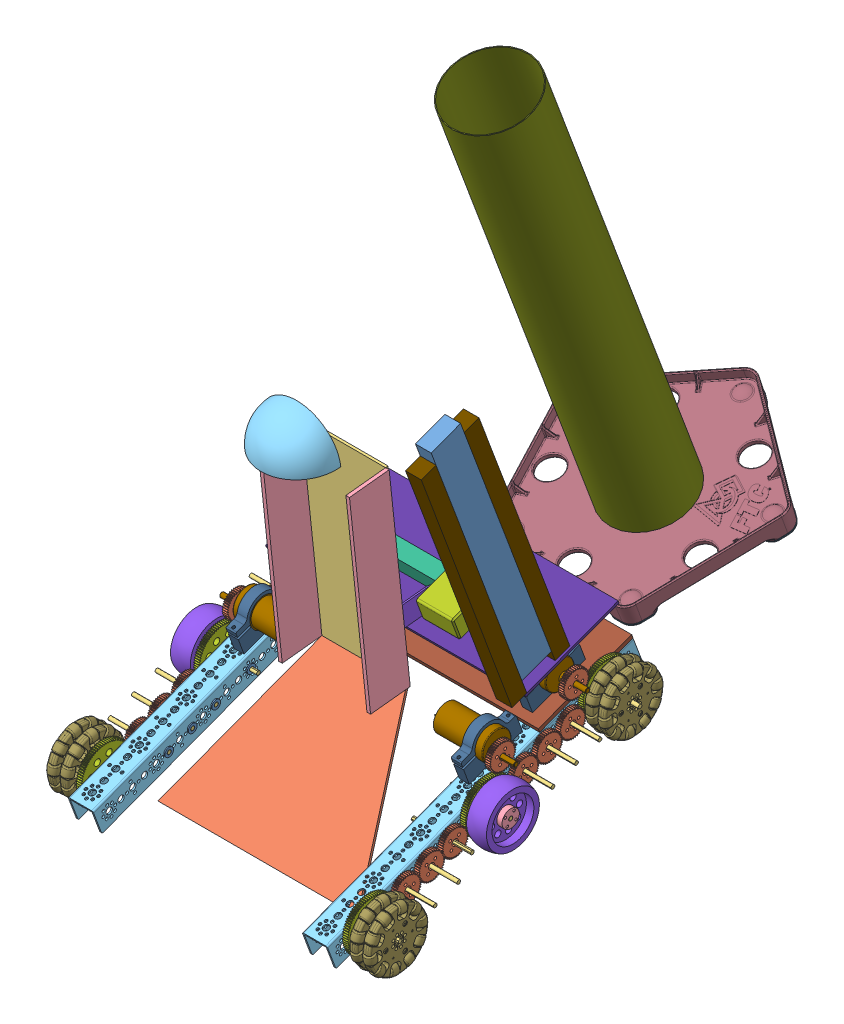
SolidWorks assembly 6157 - Basic Chassis, configuration Default. Lengths in mm.
Overall size (426.67 882.34 918.7).
152 component instances, 30 part files, 95 mates.
Components (placement in the parent):
- Part1^6157 - Basic Chassis-1: Part1^6157 - Basic Chassis [Default] at origin (virtual)
- ChassisSide^6157 - Basic Chassis-1: ChassisSide^6157 - Basic Chassis [Default] at (356.2135 -601.8803 193.3567) x (0 -0.61219 -0.790711) z (1 0 0) size (261.15 370.6 94.34) (virtual)
  - Copy of Assem7^ChassisSide_6157 - Basic Chassis-1: Copy of Assem7^ChassisSide_6157 - Basic Chassis [Default] at (59.0771 95.1521 -34.8) x (-0.863566 0.504235 0) z (0 0 -1) size (34.75 34.75 75.57) (virtual)
    - Axle bronze bushing-1: Axle bronze bushing [Default] at origin size (11 11 12.4)
    - Gear Metric 40T-1: Gear Metric 40T [PreviewCfg] at (0 0 -34.8) x (0 0 -1) z (0.99932 -0.03687 0) size (6.2 33.53 33.53)
    - Axle D-shaft-1: Axle D-shaft [Default] at (0 0 -37.7829) x (-0.991315 0.131508 0) z (0 0 1) size (4.73 4.46 75.57)
    - Axle bronze bushing-2: Axle bronze bushing [Default] at (0 0 -36.2) x (-0.381849 -0.924225 0) z (0 0 -1) size (11 11 12.4)
  - Hub axle shaft-1: Hub axle shaft [Default] at (0 0 25.25) x (-0.097328 0.995252 0) z (0 0 -1) size (22 22 9.5)
  - Pitsco Education-739069-1: Pitsco Education-739069 [Default] at (-109.4377 -176.8824 -17.4) x (0 0 1) z (-0.526143 -0.850396 0) size (32 32 416)
  - Axle bronze bushing-1: Axle bronze bushing [Default] at (-25.2548 -40.819 0) x (0.995682 -0.092835 0) z (0 0 1) size (11 11 12.4)
  - Axle bronze bushing-2: Axle bronze bushing [Default] at origin size (11 11 12.4)
  - Hub spacer-1: Hub spacer [Default] at (0 0 6.2) x (-0.466001 -0.884784 0) z (0 0 -1) size (22.2 22.2 17.7)
  - Axle D-shaft-1: Axle D-shaft [Default] at (0 0 -5.8329) x (0.055977 0.998432 0) z (0 0 1) size (4.73 4.46 75.57)
  - Gear Metric 80T-1: Gear Metric 80T [Metric - Spur gear 0.8M 80T 20PA 6.2FW ---S80N75H50L8.0N] x (0 0 1) z (-0.097328 0.995252 0) size (6.2 65.57 65.57)
  - Wheel 76mm 3-in-1: Wheel 76mm 3-in [Default] at (0 0 11.534) x (-0.995252 -0.097328 0) z (0 0 -1) size (72.2 72.2 25.4)
  - Axle bronze bushing-3: Axle bronze bushing [Default] at (0 0 -34.8) x (-0.466001 -0.884784 0) z (0 0 -1) size (11 11 12.4)
  - Axle bronze bushing-4: Axle bronze bushing [Default] at (-25.2548 -40.819 -34.8) x (-0.466001 -0.884784 0) z (0 0 -1) size (11 11 12.4)
  - Axle D-shaft-2: Axle D-shaft [Default] at (-25.2548 -40.819 -9.7171) x (0.055977 0.998432 0) z (0 0 1) size (4.73 4.46 75.57)
  - Gear Metric 40T-1: Gear Metric 40T [PreviewCfg] at (-25.2548 -40.819 0) x (0 0 1) z (0.013213 -0.999913 0) size (6.2 33.53 33.53)
  - Axle bronze bushing-5: Axle bronze bushing [Default] at (84.1828 136.0634 0) x (0.995682 -0.092835 0) z (0 0 1) size (11 11 12.4)
  - Copy of Assem7^ChassisSide_6157 - Basic Chassis-2: Copy of Assem7^ChassisSide_6157 - Basic Chassis [Default] at (-42.0914 -68.0317 -34.8) x (0.010961 -0.99994 0) z (0 0 -1) size (34.75 34.75 75.57) (virtual)
    - Axle bronze bushing-1: Axle bronze bushing [Default] at origin size (11 11 12.4)
    - Gear Metric 40T-1: Gear Metric 40T [PreviewCfg] at (0 0 -34.8) x (0 0 -1) z (0.99932 -0.03687 0) size (6.2 33.53 33.53)
    - Axle D-shaft-1: Axle D-shaft [Default] at (0 0 -37.7829) x (-0.991315 0.131508 0) z (0 0 1) size (4.73 4.46 75.57)
    - Axle bronze bushing-2: Axle bronze bushing [Default] at (0 0 -36.2) x (-0.381849 -0.924225 0) z (0 0 -1) size (11 11 12.4)
  - Gear Metric 80T-2: Gear Metric 80T [Metric - Spur gear 0.8M 80T 20PA 6.2FW ---S80N75H50L8.0N] at (84.1828 136.0634 0) x (0 0 1) z (-0.737059 -0.675828 0) size (6.2 65.57 65.57)
  - Axle D-shaft-3: Axle D-shaft [Default] at (84.1828 136.0634 9.0538) x (-0.905707 -0.423905 0) z (0 0 1) size (4.73 4.46 75.57)
  - Copy of OmniWheelGear^ChassisSide_6157 - Basic Chassis-1: Copy of OmniWheelGear^ChassisSide_6157 - Basic Chassis [Default] at (-84.1828 -136.0634 0) x (0.995682 -0.092835 0) z (0 0 1) size (92.61 92.61 75.57) (virtual)
    - Axle bronze bushing-1: Axle bronze bushing [Default] at origin size (11 11 12.4)
    - Axle bronze bushing-2: Axle bronze bushing [Default] at (0 0 -34.8) x (-0.381849 -0.924225 0) z (0 0 -1) size (11 11 12.4)
    - Axle D-shaft-1: Axle D-shaft [Default] at (0 0 2.9829) x (-0.596843 0.802358 0) z (0 0 1) size (4.73 4.46 75.57)
    - Gear Metric 80T-1: Gear Metric 80T [Metric - Spur gear 0.8M 80T 20PA 6.2FW ---S80N75H50L8.0N] x (0 0 1) z (-0.671136 -0.741335 0) size (6.2 65.57 65.57)
  - Copy of Assem7^ChassisSide_6157 - Basic Chassis-3: Copy of Assem7^ChassisSide_6157 - Basic Chassis [Default] at (-59.0771 -95.1521 -34.8) x (-0.863566 0.504235 0) z (0 0 -1) size (34.75 34.75 75.57) (virtual)
    - Axle bronze bushing-1: Axle bronze bushing [Default] at origin size (11 11 12.4)
    - Gear Metric 40T-1: Gear Metric 40T [PreviewCfg] at (0 0 -34.8) x (0 0 -1) z (0.99932 -0.03687 0) size (6.2 33.53 33.53)
    - Axle D-shaft-1: Axle D-shaft [Default] at (0 0 -37.7829) x (-0.991315 0.131508 0) z (0 0 1) size (4.73 4.46 75.57)
    - Axle bronze bushing-2: Axle bronze bushing [Default] at (0 0 -36.2) x (-0.381849 -0.924225 0) z (0 0 -1) size (11 11 12.4)
  - Copy of Assem7^ChassisSide_6157 - Basic Chassis-4: Copy of Assem7^ChassisSide_6157 - Basic Chassis [Default] at (42.0914 68.0317 -34.8) x (-0.863566 0.504235 0) z (0 0 -1) size (34.75 34.75 75.57) (virtual)
    - Axle bronze bushing-1: Axle bronze bushing [Default] at origin size (11 11 12.4)
    - Gear Metric 40T-1: Gear Metric 40T [PreviewCfg] at (0 0 -34.8) x (0 0 -1) z (0.99932 -0.03687 0) size (6.2 33.53 33.53)
    - Axle D-shaft-1: Axle D-shaft [Default] at (0 0 -37.7829) x (-0.991315 0.131508 0) z (0 0 1) size (4.73 4.46 75.57)
    - Axle bronze bushing-2: Axle bronze bushing [Default] at (0 0 -36.2) x (-0.381849 -0.924225 0) z (0 0 -1) size (11 11 12.4)
  - Copy of Assem7^ChassisSide_6157 - Basic Chassis-5: Copy of Assem7^ChassisSide_6157 - Basic Chassis [Default] at (25.2548 40.819 -34.8) x (-0.863566 0.504235 0) z (0 0 -1) size (34.75 34.75 75.57) (virtual)
    - Axle bronze bushing-1: Axle bronze bushing [Default] at origin size (11 11 12.4)
    - Gear Metric 40T-1: Gear Metric 40T [PreviewCfg] at (0 0 -34.8) x (0 0 -1) z (0.99932 -0.03687 0) size (6.2 33.53 33.53)
    - Axle D-shaft-1: Axle D-shaft [Default] at (0 0 -37.7829) x (-0.991315 0.131508 0) z (0 0 1) size (4.73 4.46 75.57)
    - Axle bronze bushing-2: Axle bronze bushing [Default] at (0 0 -36.2) x (-0.381849 -0.924225 0) z (0 0 -1) size (11 11 12.4)
- ChassisSide^6157 - Basic Chassis-2: ChassisSide^6157 - Basic Chassis [Default] at (23.2135 -601.8803 193.3567) x (0 -0.980825 0.194892) z (-1 0 0) size (261.15 370.6 94.34) (virtual)
  - Copy of Assem7^ChassisSide_6157 - Basic Chassis-1: Copy of Assem7^ChassisSide_6157 - Basic Chassis [Default] at (59.0771 95.1521 -34.8) x (-0.863566 0.504235 0) z (0 0 -1) size (34.75 34.75 75.57) (virtual)
    - Axle bronze bushing-1: Axle bronze bushing [Default] at origin size (11 11 12.4)
    - Gear Metric 40T-1: Gear Metric 40T [PreviewCfg] at (0 0 -34.8) x (0 0 -1) z (0.99932 -0.03687 0) size (6.2 33.53 33.53)
    - Axle D-shaft-1: Axle D-shaft [Default] at (0 0 -37.7829) x (-0.991315 0.131508 0) z (0 0 1) size (4.73 4.46 75.57)
    - Axle bronze bushing-2: Axle bronze bushing [Default] at (0 0 -36.2) x (-0.381849 -0.924225 0) z (0 0 -1) size (11 11 12.4)
  - Hub axle shaft-1: Hub axle shaft [Default] at (0 0 25.25) x (-0.097328 0.995252 0) z (0 0 -1) size (22 22 9.5)
  - Pitsco Education-739069-1: Pitsco Education-739069 [Default] at (-109.4377 -176.8824 -17.4) x (0 0 1) z (-0.526143 -0.850396 0) size (32 32 416)
  - Axle bronze bushing-1: Axle bronze bushing [Default] at (-25.2548 -40.819 0) x (0.995682 -0.092835 0) z (0 0 1) size (11 11 12.4)
  - Axle bronze bushing-2: Axle bronze bushing [Default] at origin size (11 11 12.4)
  - Hub spacer-1: Hub spacer [Default] at (0 0 6.2) x (-0.466001 -0.884784 0) z (0 0 -1) size (22.2 22.2 17.7)
  - Axle D-shaft-1: Axle D-shaft [Default] at (0 0 -5.8329) x (0.055977 0.998432 0) z (0 0 1) size (4.73 4.46 75.57)
  - Gear Metric 80T-1: Gear Metric 80T [Metric - Spur gear 0.8M 80T 20PA 6.2FW ---S80N75H50L8.0N] x (0 0 1) z (-0.097328 0.995252 0) size (6.2 65.57 65.57)
  - Wheel 76mm 3-in-1: Wheel 76mm 3-in [Default] at (0 0 11.534) x (-0.995252 -0.097328 0) z (0 0 -1) size (72.2 72.2 25.4)
  - Axle bronze bushing-3: Axle bronze bushing [Default] at (0 0 -34.8) x (-0.466001 -0.884784 0) z (0 0 -1) size (11 11 12.4)
  - Axle bronze bushing-4: Axle bronze bushing [Default] at (-25.2548 -40.819 -34.8) x (-0.466001 -0.884784 0) z (0 0 -1) size (11 11 12.4)
  - Axle D-shaft-2: Axle D-shaft [Default] at (-25.2548 -40.819 -9.7171) x (0.055977 0.998432 0) z (0 0 1) size (4.73 4.46 75.57)
  - Gear Metric 40T-1: Gear Metric 40T [PreviewCfg] at (-25.2548 -40.819 0) x (0 0 1) z (0.013213 -0.999913 0) size (6.2 33.53 33.53)
  - Axle bronze bushing-5: Axle bronze bushing [Default] at (84.1828 136.0634 0) x (0.995682 -0.092835 0) z (0 0 1) size (11 11 12.4)
  - Copy of Assem7^ChassisSide_6157 - Basic Chassis-2: Copy of Assem7^ChassisSide_6157 - Basic Chassis [Default] at (-42.0914 -68.0317 -34.8) x (0.010961 -0.99994 0) z (0 0 -1) size (34.75 34.75 75.57) (virtual)
    - Axle bronze bushing-1: Axle bronze bushing [Default] at origin size (11 11 12.4)
    - Gear Metric 40T-1: Gear Metric 40T [PreviewCfg] at (0 0 -34.8) x (0 0 -1) z (0.99932 -0.03687 0) size (6.2 33.53 33.53)
    - Axle D-shaft-1: Axle D-shaft [Default] at (0 0 -37.7829) x (-0.991315 0.131508 0) z (0 0 1) size (4.73 4.46 75.57)
    - Axle bronze bushing-2: Axle bronze bushing [Default] at (0 0 -36.2) x (-0.381849 -0.924225 0) z (0 0 -1) size (11 11 12.4)
  - Gear Metric 80T-2: Gear Metric 80T [Metric - Spur gear 0.8M 80T 20PA 6.2FW ---S80N75H50L8.0N] at (84.1828 136.0634 0) x (0 0 1) z (-0.737059 -0.675828 0) size (6.2 65.57 65.57)
  - Axle D-shaft-3: Axle D-shaft [Default] at (84.1828 136.0634 9.0538) x (-0.905707 -0.423905 0) z (0 0 1) size (4.73 4.46 75.57)
  - Copy of OmniWheelGear^ChassisSide_6157 - Basic Chassis-1: Copy of OmniWheelGear^ChassisSide_6157 - Basic Chassis [Default] at (-84.1828 -136.0634 0) x (0.995682 -0.092835 0) z (0 0 1) size (92.61 92.61 75.57) (virtual)
    - Axle bronze bushing-1: Axle bronze bushing [Default] at origin size (11 11 12.4)
    - Axle bronze bushing-2: Axle bronze bushing [Default] at (0 0 -34.8) x (-0.381849 -0.924225 0) z (0 0 -1) size (11 11 12.4)
    - Axle D-shaft-1: Axle D-shaft [Default] at (0 0 2.9829) x (-0.596843 0.802358 0) z (0 0 1) size (4.73 4.46 75.57)
    - Gear Metric 80T-1: Gear Metric 80T [Metric - Spur gear 0.8M 80T 20PA 6.2FW ---S80N75H50L8.0N] x (0 0 1) z (-0.671136 -0.741335 0) size (6.2 65.57 65.57)
  - Copy of Assem7^ChassisSide_6157 - Basic Chassis-3: Copy of Assem7^ChassisSide_6157 - Basic Chassis [Default] at (-59.0771 -95.1521 -34.8) x (-0.863566 0.504235 0) z (0 0 -1) size (34.75 34.75 75.57) (virtual)
    - Axle bronze bushing-1: Axle bronze bushing [Default] at origin size (11 11 12.4)
    - Gear Metric 40T-1: Gear Metric 40T [PreviewCfg] at (0 0 -34.8) x (0 0 -1) z (0.99932 -0.03687 0) size (6.2 33.53 33.53)
    - Axle D-shaft-1: Axle D-shaft [Default] at (0 0 -37.7829) x (-0.991315 0.131508 0) z (0 0 1) size (4.73 4.46 75.57)
    - Axle bronze bushing-2: Axle bronze bushing [Default] at (0 0 -36.2) x (-0.381849 -0.924225 0) z (0 0 -1) size (11 11 12.4)
  - Copy of Assem7^ChassisSide_6157 - Basic Chassis-4: Copy of Assem7^ChassisSide_6157 - Basic Chassis [Default] at (42.0914 68.0317 -34.8) x (-0.863566 0.504235 0) z (0 0 -1) size (34.75 34.75 75.57) (virtual)
    - Axle bronze bushing-1: Axle bronze bushing [Default] at origin size (11 11 12.4)
    - Gear Metric 40T-1: Gear Metric 40T [PreviewCfg] at (0 0 -34.8) x (0 0 -1) z (0.99932 -0.03687 0) size (6.2 33.53 33.53)
    - Axle D-shaft-1: Axle D-shaft [Default] at (0 0 -37.7829) x (-0.991315 0.131508 0) z (0 0 1) size (4.73 4.46 75.57)
    - Axle bronze bushing-2: Axle bronze bushing [Default] at (0 0 -36.2) x (-0.381849 -0.924225 0) z (0 0 -1) size (11 11 12.4)
  - Copy of Assem7^ChassisSide_6157 - Basic Chassis-5: Copy of Assem7^ChassisSide_6157 - Basic Chassis [Default] at (25.2548 40.819 -34.8) x (-0.863566 0.504235 0) z (0 0 -1) size (34.75 34.75 75.57) (virtual)
    - Axle bronze bushing-1: Axle bronze bushing [Default] at origin size (11 11 12.4)
    - Gear Metric 40T-1: Gear Metric 40T [PreviewCfg] at (0 0 -34.8) x (0 0 -1) z (0.99932 -0.03687 0) size (6.2 33.53 33.53)
    - Axle D-shaft-1: Axle D-shaft [Default] at (0 0 -37.7829) x (-0.991315 0.131508 0) z (0 0 1) size (4.73 4.46 75.57)
    - Axle bronze bushing-2: Axle bronze bushing [Default] at (0 0 -36.2) x (-0.381849 -0.924225 0) z (0 0 -1) size (11 11 12.4)
- UseFF42-1: UseFF42 [Default] at (54.9635 -516.2212 88.7348) x (0 0.791255 -0.611486) z (0 0.611486 0.791255) size (37 98.8 37)
- Pitsco Education-739089-1: Pitsco Education-739089 [Default] at (42.664 -512.4253 78.2601) x (0 -0.350318 0.936631) z (-1 0 0) size (72 44.98 12.7)
- Pitsco Education-739089-3: Pitsco Education-739089 [Default] at (52.223 -556.6367 181.9652) x (0 0.350318 -0.936631) z (1 0 0) size (72 44.98 12.7)
- UseFF42-2: UseFF42 [Default] at (52.6235 -552.627 171.5704) x (0 -0.24033 -0.970691) z (0 0.970691 -0.24033) size (37 98.8 37)
- Pitsco Education-739089-4: Pitsco Education-739089 [Default] at (339.103 -556.6367 181.9652) x (0 0.350318 -0.936631) z (1 0 0) size (72 44.98 12.7)
- Pitsco Education-739089-5: Pitsco Education-739089 [Default] at (324.864 -512.4253 78.2601) x (0 -0.350318 0.936631) z (-1 0 0) size (72 44.98 12.7)
- UseFF42-3: UseFF42 [Default] at (324.4635 -516.2212 88.7348) x (0 -0.689259 0.724515) z (0 0.724515 0.689259) size (37 98.8 37)
- UseFF42-4: UseFF42 [Default] at (326.8035 -552.627 171.5704) x (0 0.965735 0.25953) z (0 0.25953 -0.965735) size (37 98.8 37)
- Part11^6157 - Basic Chassis-1: Part11^6157 - Basic Chassis [Default] at origin (virtual)
- Part12^6157 - Basic Chassis-1: Part12^6157 - Basic Chassis [Default] at origin (virtual)
- SheetMetalBack-1: SheetMetalBack [Default] at (268.8694 -537.4577 66.7854) x (0 0.350318 -0.936631) z (1 0 0) size (127 5.08 330.2)
- Gear Metric 40T-2: Gear Metric 40T [PreviewCfg] at (356.2135 -554.314 177.8477) x (1 0 0) z (0 -0.911719 0.410815) size (6.2 33.53 33.53)
- Gear Metric 40T-3: Gear Metric 40T [PreviewCfg] at (356.2135 -520.9306 84.2546) x (1 0 0) z (0 -0.059742 -0.998214) size (6.2 33.53 33.53)
- Gear Metric 40T-4: Gear Metric 40T [PreviewCfg] at (17.0135 -520.1959 83.5917) x (1 0 0) z (0 -0.298109 0.954532) size (6.2 33.53 33.53)
- Gear Metric 40T-5: Gear Metric 40T [PreviewCfg] at (17.0135 -558.9365 173.1326) x (1 0 0) z (0 0.678187 0.734889) size (6.2 33.53 33.53)
- 3-inch omni single wheel part-1: 3-inch omni single wheel part [Default] at (376.988 -664.2337 340.0098) x (0 -0.888989 -0.457929) z (0 0.457929 -0.888989) size (77.7 13.48 77.72)
- Hub axle shaft-1: Hub axle shaft [Default] at (362.4135 -657.9312 343.2176) x (0 0.442694 -0.896673) z (-1 0 0) size (22 22 9.5)
- Hub axle shaft-2: Hub axle shaft [Default] at (379.1135 -657.9312 343.2176) x (0 0.442694 -0.896673) z (-1 0 0) size (22 22 9.5)
- 3-inch omni single wheel part-2: 3-inch omni single wheel part [Default] at (393.688 -651.2061 341.0302) x (0 0.952454 -0.304681) z (0 0.304681 0.952454) size (77.7 13.48 77.72)
- 3-inch omni single wheel part-4: 3-inch omni single wheel part [Default] at (393.688 -539.1043 41.3083) x (0 0.952454 -0.304681) z (0 0.304681 0.952454) size (77.7 13.48 77.72)
- Hub axle shaft-3: Hub axle shaft [Default] at (362.4135 -545.8294 43.4958) x (0 0.442694 -0.896673) z (-1 0 0) size (22 22 9.5)
- 3-inch omni single wheel part-5: 3-inch omni single wheel part [Default] at (376.988 -552.132 40.288) x (0 -0.888989 -0.457929) z (0 0.457929 -0.888989) size (77.7 13.48 77.72)
- Hub axle shaft-4: Hub axle shaft [Default] at (379.1135 -545.8294 43.4958) x (0 0.442694 -0.896673) z (-1 0 0) size (22 22 9.5)
- 3-inch omni single wheel part-6: 3-inch omni single wheel part [Default] at (-14.261 -662.5209 348.5979) x (0 -0.645288 0.763939) z (0 0.763939 0.645288) size (77.7 13.48 77.72)
- Hub axle shaft-5: Hub axle shaft [Default] at (17.0135 -657.9312 343.2176) x (0 0.997769 -0.066755) z (1 0 0) size (22 22 9.5)
- 3-inch omni single wheel part-7: 3-inch omni single wheel part [Default] at (2.439 -658.4893 336.1678) x (0 -0.08377 -0.996485) z (0 -0.996485 0.08377) size (77.7 13.48 77.72)
- Hub axle shaft-6: Hub axle shaft [Default] at (0.3135 -657.9312 343.2176) x (0 0.997769 -0.066755) z (1 0 0) size (22 22 9.5)
- Hub axle shaft-9: Hub axle shaft [Default] at (0.3135 -545.8294 43.4958) x (0 0.997769 -0.066755) z (1 0 0) size (22 22 9.5)
- 3-inch omni single wheel part-10: 3-inch omni single wheel part [Default] at (2.439 -546.3875 36.4459) x (0 -0.08377 -0.996485) z (0 -0.996485 0.08377) size (77.7 13.48 77.72)
- 3-inch omni single wheel part-11: 3-inch omni single wheel part [Default] at (-14.261 -550.4191 48.876) x (0 -0.645288 0.763939) z (0 0.763939 0.645288) size (77.7 13.48 77.72)
- Hub axle shaft-10: Hub axle shaft [Default] at (17.0135 -545.8294 43.4958) x (0 0.997769 -0.066755) z (1 0 0) size (22 22 9.5)
- Rolling_Goal-60cm-1: Rolling_Goal-60cm [Default] at (207.5611 -534.7556 -157.3658) x (0.309017 -0.333172 0.890789) z (-0.951057 -0.108254 0.289435) size (291.98 600.59 285.9)
  - Final Rev1-2 - Pentagon Base-1: Final Rev1-2 - Pentagon Base [Default] at (-9.8868 20.1576 -8.4777) size (283.35 51.39 274.75)
  - Final Rev1 - Pentagon Foot-1: Final Rev1 - Pentagon Foot [Default] at (-84.6377 13.8076 94.5082) x (0.809017 0 -0.587785) z (0.587785 0 0.809017) size (40.81 17.65 43.23)
  - 1in Ball Caster-1: 1in Ball Caster [Default] at (-85.3501 20.1576 95.3886) size (25.4 25.4 25.4)
  - Final Rev1 - Pentagon Foot-2: Final Rev1 - Pentagon Foot [Default] at (64.9593 13.8076 94.439) x (-0.309017 0 -0.951057) z (0.951057 0 -0.309017) size (40.81 17.65 43.23)
  - Final Rev1 - Pentagon Foot-3: Final Rev1 - Pentagon Foot [Default] at (111.1214 13.8076 -47.8575) x (-1 0 0) z (0 0 -1) size (40.81 17.65 43.23)
  - Final Rev1 - Pentagon Foot-4: Final Rev1 - Pentagon Foot [Default] at (-9.9457 13.8076 -135.7324) x (-0.309017 0 0.951057) z (-0.951057 0 -0.309017) size (40.81 17.65 43.23)
  - Final Rev1 - Pentagon Foot-5: Final Rev1 - Pentagon Foot [Default] at (-130.9315 13.8076 -47.7455) x (0.809017 0 0.587785) z (-0.587785 0 0.809017) size (40.81 17.65 43.23)
  - 1in Ball Caster-2: 1in Ball Caster [Default] at (65.5764 20.1576 95.3886) x (0.309017 0 -0.951057) z (0.951057 0 0.309017) size (25.4 25.4 25.4)
  - 1in Ball Caster-3: 1in Ball Caster [Default] at (112.2152 20.1576 -48.151) x (-0.809017 0 -0.587785) z (0.587785 0 -0.809017) size (25.4 25.4 25.4)
  - 1in Ball Caster-4: 1in Ball Caster [Default] at (-9.8868 20.1576 -136.8634) x (-0.809017 0 0.587785) z (-0.587785 0 -0.809017) size (25.4 25.4 25.4)
  - 1in Ball Caster-5: 1in Ball Caster [Default] at (-131.9889 20.1576 -48.151) x (0.309017 0 0.951057) z (-0.951057 0 0.309017) size (25.4 25.4 25.4)
  - Pipe - 60cm-1: Pipe - 60cm [Default] at (-9.8868 32.8576 -8.4777) size (103.63 574.6 103.63)
- top plate-1: top plate [Default] at (24.6135 -510.8275 140.932) x (1 0 0) z (0 0.936631 0.350318) size (330.2 127 3.17)
- 20x20Piece-1: 20x20Piece [Default] at (354.8135 -513.9239 158.2738) x (-1 0 0) z (0 0.936631 0.350318) size (20 20 330.2)
- 20x20Piece-2: 20x20Piece [Default] at (354.8135 -489.1824 103.4682) x (-1 0 0) z (0 0.936631 0.350318) size (20 20 330.2)
- 20 by 40 peace-1: 20 by 40 peace [Default] at (354.8135 -476.5639 108.1878) x (-1 0 0) z (0 0.350318 -0.936631) size (20 330.2 40)
- Assem1^6157 - Basic Chassis-1: Assem1^6157 - Basic Chassis [Default] at origin (virtual)
- dustpan-1: dustpan [Default] at (112.0693 -616.6979 597.1087) x (-1 0 0) z (0 -0.66823 -0.743955) size (254 390.64 321.26)
  - Dustpan_trapazoid-1: Dustpan_trapazoid [Default] at (-153.1614 342.3354 222.2504) size (254 203.2 3.17)
  - dustpan_dispense-1: dustpan_dispense [Default] at (-153.1614 514.654 35.6161) x (0 -0.669131 0.743145) z (1 0 0) size (254 3.17 107.95)
  - Part1^dustpan-1: Part1^dustpan [Default] at (-153.1614 514.654 35.6161) x (0 0.669131 -0.743145) z (-1 0 0) (virtual)
  - Part2^dustpan-1: Part2^dustpan [Default] at (-153.1614 570.9718 32.3937) x (0 0.669131 -0.743145) z (-1 0 0) size (254 50.8 4.57) (virtual)
  - Part2^dustpan-2: Part2^dustpan [Default] at (-45.2114 469.5012 -58.9708) x (0 0.669131 -0.743145) z (1 0 0) size (254 50.8 4.57) (virtual)
  - Part3^dustpan-1: Part3^dustpan [Default] at (-153.1614 495.7877 -24.0951) x (0 -0.669131 0.743145) z (0 -0.743145 -0.669131) size (50.8 101.6 50.8) (virtual)
- Part2^6157 - Basic Chassis-1: Part2^6157 - Basic Chassis [Default] at (334.8135 -489.1824 103.4682) x (0 -0.936631 -0.350318) z (-1 0 0) size (20.02 20 279.4) (virtual)
- QuarterScaleServo-1: QuarterScaleServo [Default] at (277.5727 -452.1223 130.0041) x (0 -0.350318 0.936631) z (0 -0.936631 -0.350318) size (59.05 50.29 28.45)
- QuarterScaleServoMountArm-1: QuarterScaleServoMountArm [Default] at (-232.1052 -449.4532 -146.3135) x (0 0.105733 -0.994395) z (1 0 0) size (77.5 27 72)
Mates (geometry in assembly coordinates):
- Concentric77: concentric aligned: cylinder of ChassisSide^6157 - Basic Chassis-2/Pitsco Education-739069-1 through (46.2735 -592.4632 122.5059) axis (0 0.936631 0.350318) radius 1.85; cylinder of Pitsco Education-739089-3 through (46.2735 -562.491 133.7161) axis (0 0.936631 0.350318) radius 1.85
- Concentric78: concentric aligned: cylinder of ChassisSide^6157 - Basic Chassis-2/Pitsco Education-739069-1 through (46.2735 -614.8836 182.4503) axis (0 0.936631 0.350318) radius 1.85; cylinder of Pitsco Education-739089-3 through (46.2735 -584.9114 193.6605) axis (0 0.936631 0.350318) radius 1.85
- Coincident63: coincident anti-aligned: plane of ChassisSide^6157 - Basic Chassis-2/Pitsco Education-739069-1 through (56.6135 -659.7603 393.781) normal (0 0.936631 0.350318); plane of Pitsco Education-739089-3 through (39.9235 -586.3127 197.407) normal (0 -0.936631 -0.350318)
- Concentric80: concentric anti-aligned: cylinder of UseFF42-1 through (99.4635 -516.2212 88.7348) axis (1 0 0) radius 18.5; cylinder of Pitsco Education-739089-1 through (54.9635 -516.2212 88.7348) axis (-1 0 0) radius 18.5
- Coincident64: coincident aligned: plane of UseFF42-1 through (54.9635 -502.7699 78.3396) normal (1 0 0); plane of Pitsco Education-739089-1 through (54.9635 -516.2212 88.7348) normal (1 0 0)
- Concentric82: concentric aligned: cylinder of Pitsco Education-739089-3 through (39.9235 -552.627 171.5704) axis (1 0 0) radius 18.5; cylinder of UseFF42-2 through (97.1235 -552.627 171.5704) axis (1 0 0) radius 18.5
- Coincident65: coincident aligned: plane of Pitsco Education-739089-3 through (52.6235 -552.627 171.5704) normal (1 0 0); circle of UseFF42-2
- Coincident66: coincident aligned: circle of ChassisSide^6157 - Basic Chassis-1/Pitsco Education-739069-1; cylinder of Pitsco Education-739089-4 through (333.1535 -562.491 133.7161) axis (0 0.936631 0.350318) radius 1.85
- Concentric83: concentric aligned: cylinder of ChassisSide^6157 - Basic Chassis-1/Pitsco Education-739069-1 through (333.1535 -614.8836 182.4503) axis (0 0.936631 0.350318) radius 1.85; cylinder of Pitsco Education-739089-4 through (333.1535 -584.9114 193.6605) axis (0 0.936631 0.350318) radius 1.85
- Coincident67: coincident anti-aligned: plane of ChassisSide^6157 - Basic Chassis-1/Pitsco Education-739069-1 through (322.8135 -514.028 4.1426) normal (0 0.936631 0.350318); plane of Pitsco Education-739089-4 through (326.8035 -586.3127 197.407) normal (0 -0.936631 -0.350318)
- Concentric85: concentric aligned: cylinder of Pitsco Education-739089-5 through (337.1635 -516.2212 88.7348) axis (-1 0 0) radius 18.5; cylinder of UseFF42-3 through (279.9635 -516.2212 88.7348) axis (-1 0 0) radius 18.5
- Coincident71: coincident aligned: plane of Pitsco Education-739089-5 through (324.4635 -516.2212 88.7348) normal (-1 0 0); circle of UseFF42-3
- Concentric86: concentric anti-aligned: cylinder of Pitsco Education-739089-4 through (326.8035 -552.627 171.5704) axis (1 0 0) radius 18.5; cylinder of UseFF42-4 through (282.3035 -552.627 171.5704) axis (-1 0 0) radius 18.5
- Coincident72: coincident aligned: plane of Pitsco Education-739089-4 through (326.8035 -552.627 171.5704) normal (-1 0 0); circle of UseFF42-4
- Coincident82: coincident aligned: plane of ChassisSide^6157 - Basic Chassis-1/Pitsco Education-739069-1 through (354.8135 -514.028 4.1426) normal (1 0 0); plane of SheetMetalBack-1 through (354.8135 -553.7604 124.8743) normal (1 0 0)
- Coincident83: coincident aligned: plane of ChassisSide^6157 - Basic Chassis-2/Pitsco Education-739069-1 through (24.6135 -659.7603 393.781) normal (-1 0 0); plane of SheetMetalBack-1 through (24.6135 -553.7604 124.8743) normal (-1 0 0)
- Coincident84: coincident aligned: plane of ChassisSide^6157 - Basic Chassis-1/Pitsco Education-739069-1 through (338.8135 -529.0141 -1.4625) normal (0 0.350318 -0.936631); plane of SheetMetalBack-1 through (24.6135 -509.27 5.9222) normal (0 0.350318 -0.936631)
- Coincident85: coincident aligned: plane of ChassisSide^6157 - Basic Chassis-2/Pitsco Education-739069-1 through (40.6135 -529.0141 -1.4625) normal (0 0.350318 -0.936631); plane of SheetMetalBack-1 through (24.6135 -509.27 5.9222) normal (0 0.350318 -0.936631)
- Coincident86: coincident anti-aligned: plane of ChassisSide^6157 - Basic Chassis-2/Pitsco Education-739069-1 through (56.6135 -659.7603 393.781) normal (0 0.936631 0.350318); plane of SheetMetalBack-1 through (268.8694 -537.4577 66.7854) normal (0 -0.936631 -0.350318)
- Coincident87: coincident anti-aligned: plane of ChassisSide^6157 - Basic Chassis-1/Pitsco Education-739069-1 through (322.8135 -514.028 4.1426) normal (0 0.936631 0.350318); plane of SheetMetalBack-1 through (268.8694 -537.4577 66.7854) normal (0 -0.936631 -0.350318)
- Concentric87: concentric aligned: cylinder of ChassisSide^6157 - Basic Chassis-1/Pitsco Education-739069-1 through (330.8135 -583.2359 97.835) axis (0 0.936631 0.350318) radius 1.85; cylinder of Pitsco Education-739089-5 through (330.8135 -548.5056 110.8248) axis (0 0.936631 0.350318) radius 1.85
- Concentric88: concentric aligned: cylinder of ChassisSide^6157 - Basic Chassis-1/Pitsco Education-739069-1 through (330.8135 -560.8155 37.8907) axis (0 0.936631 0.350318) radius 1.85; cylinder of Pitsco Education-739089-5 through (330.8135 -526.0852 50.8805) axis (0 0.936631 0.350318) radius 1.85
- Coincident88: coincident anti-aligned: plane of Pitsco Education-739089-5 through (337.1635 -524.684 47.1339) normal (0 -0.936631 -0.350318); plane of SheetMetalBack-1 through (268.8694 -532.6996 68.565) normal (0 0.936631 0.350318)
- Concentric89: concentric anti-aligned: cylinder of UseFF42-4 through (379.6035 -554.314 177.8477) axis (1 0 0) radius 3; cylinder of Gear Metric 40T-2 through (406.2135 -554.314 177.8477) axis (-1 0 0) radius 4
- Coincident89: coincident aligned: plane of ChassisSide^6157 - Basic Chassis-1/Gear Metric 80T-1 through (362.4135 -601.8803 193.3567) normal (1 0 0); plane of Gear Metric 40T-2 through (362.4135 -554.314 177.8477) normal (1 0 0)
- Concentric90: concentric anti-aligned: cylinder of UseFF42-3 through (377.2635 -520.9306 84.2546) axis (1 0 0) radius 3; circle of Gear Metric 40T-3
- Coincident90: coincident aligned: plane of ChassisSide^6157 - Basic Chassis-1/Gear Metric 80T-2 through (362.4135 -545.8294 43.4958) normal (1 0 0); plane of Gear Metric 40T-3 through (362.4135 -520.9306 84.2546) normal (1 0 0)
- Concentric91: concentric aligned: cylinder of ChassisSide^6157 - Basic Chassis-2/Pitsco Education-739069-1 through (48.6135 -583.2359 97.835) axis (0 0.936631 0.350318) radius 1.85; cylinder of Pitsco Education-739089-1 through (48.6135 -548.5056 110.8248) axis (0 0.936631 0.350318) radius 1.85
- Concentric92: concentric aligned: cylinder of ChassisSide^6157 - Basic Chassis-2/Pitsco Education-739069-1 through (48.6135 -560.8155 37.8907) axis (0 0.936631 0.350318) radius 1.85; cylinder of Pitsco Education-739089-1 through (48.6135 -526.0852 50.8805) axis (0 0.936631 0.350318) radius 1.85
- Coincident91: coincident anti-aligned: plane of Pitsco Education-739089-1 through (54.9635 -524.684 47.1339) normal (0 -0.936631 -0.350318); plane of SheetMetalBack-1 through (268.8694 -532.6996 68.565) normal (0 0.936631 0.350318)
- Concentric93: concentric aligned: cylinder of UseFF42-1 through (2.1635 -520.1959 83.5917) axis (-1 0 0) radius 3; cylinder of Gear Metric 40T-4 through (67.0135 -520.1959 83.5917) axis (-1 0 0) radius 4
- Coincident92: coincident aligned: plane of ChassisSide^6157 - Basic Chassis-2/Copy of OmniWheelGear^ChassisSide_6157 - Basic Chassis-1/Gear Metric 80T-1 through (17.0135 -545.8294 43.4958) normal (-1 0 0); plane of Gear Metric 40T-4 through (17.0135 -520.1959 83.5917) normal (-1 0 0)
- Coincident93: coincident aligned: plane of ChassisSide^6157 - Basic Chassis-2/Gear Metric 40T-1 through (17.0135 -585.065 148.3984) normal (-1 0 0); plane of Gear Metric 40T-5 through (17.0135 -558.9365 173.1326) normal (-1 0 0)
- Concentric94: concentric aligned: cylinder of UseFF42-2 through (-0.1765 -558.9365 173.1326) axis (-1 0 0) radius 3; cylinder of Gear Metric 40T-5 through (67.0135 -558.9365 173.1326) axis (-1 0 0) radius 4
- Concentric95: concentric anti-aligned: cylinder of ChassisSide^6157 - Basic Chassis-1/Copy of OmniWheelGear^ChassisSide_6157 - Basic Chassis-1/Axle D-shaft-1 through (321.4135 -657.9312 343.2176) axis (1 0 0) radius 2.365; cylinder of 3-inch omni single wheel part-1 through (374.1135 -657.9312 343.2176) axis (-1 0 0) radius 4
- Concentric99: concentric anti-aligned: cylinder of ChassisSide^6157 - Basic Chassis-1/Copy of OmniWheelGear^ChassisSide_6157 - Basic Chassis-1/Axle D-shaft-1 through (321.4135 -657.9312 343.2176) axis (1 0 0) radius 2.365; cylinder of Hub axle shaft-1 through (369.1135 -657.9312 343.2176) axis (-1 0 0) radius 2.3495
- Coincident96: coincident anti-aligned: plane of ChassisSide^6157 - Basic Chassis-1/Copy of OmniWheelGear^ChassisSide_6157 - Basic Chassis-1/Gear Metric 80T-1 through (362.4135 -657.9312 343.2176) normal (1 0 0); plane of Hub axle shaft-1 through (362.4135 -657.9312 343.2176) normal (-1 0 0)
- Coincident97: coincident anti-aligned: plane of 3-inch omni single wheel part-1 through (369.1135 -635.2899 329.1706) normal (-1 0 0); plane of Hub axle shaft-1 through (369.1135 -657.9312 343.2176) normal (1 0 0)
- Concentric100: concentric anti-aligned: cylinder of ChassisSide^6157 - Basic Chassis-1/Copy of OmniWheelGear^ChassisSide_6157 - Basic Chassis-1/Axle D-shaft-1 through (321.4135 -657.9312 343.2176) axis (1 0 0) radius 2.365; cylinder of Hub axle shaft-2 through (385.8135 -657.9312 343.2176) axis (-1 0 0) radius 2.3495
- Coincident98: coincident anti-aligned: plane of 3-inch omni single wheel part-1 through (379.1135 -667.8306 318.48) normal (1 0 0); plane of Hub axle shaft-2 through (379.1135 -657.9312 343.2176) normal (-1 0 0)
- Concentric101: concentric aligned: cylinder of ChassisSide^6157 - Basic Chassis-1/Copy of OmniWheelGear^ChassisSide_6157 - Basic Chassis-1/Axle D-shaft-1 through (321.4135 -657.9312 343.2176) axis (1 0 0) radius 2.365; cylinder of 3-inch omni single wheel part-2 through (390.8135 -657.9312 343.2176) axis (1 0 0) radius 4
- Coincident99: coincident anti-aligned: plane of Hub axle shaft-2 through (385.8135 -657.9312 343.2176) normal (1 0 0); plane of 3-inch omni single wheel part-2 through (385.8135 -664.0115 369.1594) normal (-1 0 0)
- Concentric102: concentric aligned: cylinder of 3-inch omni single wheel part-1 through (374.1135 -661.5389 336.0773) axis (1 0 0) radius 1.8; cylinder of 3-inch omni single wheel part-2 through (390.8135 -661.5389 336.0773) axis (1 0 0) radius 1.8
- Coincident100: coincident anti-aligned: plane of Hub axle shaft-3 through (369.1135 -545.8294 43.4958) normal (1 0 0); plane of 3-inch omni single wheel part-5 through (369.1135 -523.1882 29.4487) normal (-1 0 0)
- Coincident101: coincident anti-aligned: plane of 3-inch omni single wheel part-5 through (379.1135 -555.7288 18.7582) normal (1 0 0); plane of Hub axle shaft-4 through (379.1135 -545.8294 43.4958) normal (-1 0 0)
- Coincident102: coincident anti-aligned: plane of 3-inch omni single wheel part-4 through (385.8135 -551.9098 69.4375) normal (-1 0 0); plane of Hub axle shaft-4 through (385.8135 -545.8294 43.4958) normal (1 0 0)
- Concentric103: concentric aligned: cylinder of 3-inch omni single wheel part-4 through (390.8135 -549.4371 36.3554) axis (1 0 0) radius 1.8; cylinder of 3-inch omni single wheel part-5 through (374.1135 -549.4371 36.3554) axis (1 0 0) radius 1.8
- Concentric104: concentric anti-aligned: cylinder of ChassisSide^6157 - Basic Chassis-1/Axle D-shaft-3 through (327.4844 -545.8294 43.4958) axis (1 0 0) radius 2.365; cylinder of 3-inch omni single wheel part-5 through (374.1135 -545.8294 43.4958) axis (-1 0 0) radius 4
- Coincident103: coincident anti-aligned: plane of ChassisSide^6157 - Basic Chassis-1/Gear Metric 80T-2 through (362.4135 -545.8294 43.4958) normal (1 0 0); plane of Hub axle shaft-3 through (362.4135 -545.8294 43.4958) normal (-1 0 0)
- Concentric105: concentric anti-aligned: cylinder of ChassisSide^6157 - Basic Chassis-1/Axle D-shaft-3 through (327.4844 -545.8294 43.4958) axis (1 0 0) radius 2.365; cylinder of Hub axle shaft-4 through (385.8135 -545.8294 43.4958) axis (-1 0 0) radius 2.3495
- Concentric106: concentric aligned: cylinder of ChassisSide^6157 - Basic Chassis-1/Axle D-shaft-3 through (327.4844 -545.8294 43.4958) axis (1 0 0) radius 2.365; cylinder of 3-inch omni single wheel part-4 through (390.8135 -545.8294 43.4958) axis (1 0 0) radius 4
- Concentric107: concentric anti-aligned: cylinder of ChassisSide^6157 - Basic Chassis-1/Axle D-shaft-3 through (327.4844 -545.8294 43.4958) axis (1 0 0) radius 2.365; cylinder of Hub axle shaft-3 through (369.1135 -545.8294 43.4958) axis (-1 0 0) radius 2.3495
- Coincident104: coincident anti-aligned: plane of Hub axle shaft-5 through (10.3135 -657.9312 343.2176) normal (-1 0 0); plane of 3-inch omni single wheel part-7 through (10.3135 -679.5594 358.7794) normal (1 0 0)
- Coincident105: coincident anti-aligned: plane of 3-inch omni single wheel part-7 through (0.3135 -677.0142 324.6223) normal (-1 0 0); plane of Hub axle shaft-6 through (0.3135 -657.9312 343.2176) normal (1 0 0)
- Coincident106: coincident anti-aligned: plane of 3-inch omni single wheel part-6 through (-6.3865 -631.6334 347.5039) normal (1 0 0); plane of Hub axle shaft-6 through (-6.3865 -657.9312 343.2176) normal (-1 0 0)
- Concentric108: concentric aligned: cylinder of 3-inch omni single wheel part-6 through (-11.3865 -663.1528 337.1567) axis (-1 0 0) radius 1.8; cylinder of 3-inch omni single wheel part-7 through (5.3135 -663.1528 337.1567) axis (-1 0 0) radius 1.8
- Concentric109: concentric anti-aligned: cylinder of ChassisSide^6157 - Basic Chassis-2/Axle D-shaft-3 through (51.9426 -657.9312 343.2176) axis (-1 0 0) radius 2.365; cylinder of 3-inch omni single wheel part-7 through (5.3135 -657.9312 343.2176) axis (1 0 0) radius 4
- Concentric110: concentric anti-aligned: cylinder of ChassisSide^6157 - Basic Chassis-2/Axle D-shaft-3 through (51.9426 -657.9312 343.2176) axis (-1 0 0) radius 2.365; cylinder of Hub axle shaft-5 through (10.3135 -657.9312 343.2176) axis (1 0 0) radius 2.3495
- Coincident107: coincident anti-aligned: plane of ChassisSide^6157 - Basic Chassis-2/Gear Metric 80T-2 through (17.0135 -657.9312 343.2176) normal (-1 0 0); plane of Hub axle shaft-5 through (17.0135 -657.9312 343.2176) normal (1 0 0)
- Concentric111: concentric anti-aligned: cylinder of ChassisSide^6157 - Basic Chassis-2/Axle D-shaft-3 through (51.9426 -657.9312 343.2176) axis (-1 0 0) radius 2.365; cylinder of Hub axle shaft-6 through (-6.3865 -657.9312 343.2176) axis (1 0 0) radius 2.3495
- Concentric112: concentric aligned: cylinder of ChassisSide^6157 - Basic Chassis-2/Axle D-shaft-3 through (51.9426 -657.9312 343.2176) axis (-1 0 0) radius 2.365; cylinder of 3-inch omni single wheel part-6 through (-11.3865 -657.9312 343.2176) axis (-1 0 0) radius 4
- Coincident112: coincident anti-aligned: plane of 3-inch omni single wheel part-10 through (10.3135 -567.4576 59.0575) normal (1 0 0); plane of Hub axle shaft-10 through (10.3135 -545.8294 43.4958) normal (-1 0 0)
- Coincident113: coincident anti-aligned: plane of Hub axle shaft-9 through (0.3135 -545.8294 43.4958) normal (1 0 0); plane of 3-inch omni single wheel part-10 through (0.3135 -564.9124 24.9005) normal (-1 0 0)
- Coincident114: coincident anti-aligned: plane of Hub axle shaft-9 through (-6.3865 -545.8294 43.4958) normal (-1 0 0); plane of 3-inch omni single wheel part-11 through (-6.3865 -519.5316 47.782) normal (1 0 0)
- Concentric118: concentric aligned: cylinder of 3-inch omni single wheel part-10 through (5.3135 -551.0511 37.4349) axis (-1 0 0) radius 1.8; cylinder of 3-inch omni single wheel part-11 through (-11.3865 -551.0511 37.4349) axis (-1 0 0) radius 1.8
- Concentric119: concentric anti-aligned: cylinder of ChassisSide^6157 - Basic Chassis-2/Copy of OmniWheelGear^ChassisSide_6157 - Basic Chassis-1/Axle D-shaft-1 through (58.0135 -545.8294 43.4958) axis (-1 0 0) radius 2.365; cylinder of 3-inch omni single wheel part-10 through (5.3135 -545.8294 43.4958) axis (1 0 0) radius 4
- Concentric120: concentric anti-aligned: cylinder of ChassisSide^6157 - Basic Chassis-2/Copy of OmniWheelGear^ChassisSide_6157 - Basic Chassis-1/Axle D-shaft-1 through (58.0135 -545.8294 43.4958) axis (-1 0 0) radius 2.365; cylinder of Hub axle shaft-10 through (10.3135 -545.8294 43.4958) axis (1 0 0) radius 2.3495
- Coincident115: coincident anti-aligned: plane of ChassisSide^6157 - Basic Chassis-2/Copy of OmniWheelGear^ChassisSide_6157 - Basic Chassis-1/Gear Metric 80T-1 through (17.0135 -545.8294 43.4958) normal (-1 0 0); plane of Hub axle shaft-10 through (17.0135 -545.8294 43.4958) normal (1 0 0)
- Concentric121: concentric anti-aligned: cylinder of ChassisSide^6157 - Basic Chassis-2/Copy of OmniWheelGear^ChassisSide_6157 - Basic Chassis-1/Axle D-shaft-1 through (58.0135 -545.8294 43.4958) axis (-1 0 0) radius 2.365; cylinder of Hub axle shaft-9 through (-6.3865 -545.8294 43.4958) axis (1 0 0) radius 2.3495
- Concentric122: concentric aligned: cylinder of ChassisSide^6157 - Basic Chassis-2/Copy of OmniWheelGear^ChassisSide_6157 - Basic Chassis-1/Axle D-shaft-1 through (58.0135 -545.8294 43.4958) axis (-1 0 0) radius 2.365; cylinder of 3-inch omni single wheel part-11 through (-11.3865 -545.8294 43.4958) axis (-1 0 0) radius 4
- Coincident117: coincident aligned: plane of SheetMetalBack-1 through (24.6135 -509.27 5.9222) normal (0 0.350318 -0.936631); plane of top plate-1 through (24.6135 -463.3633 23.0922) normal (0 0.350318 -0.936631)
- Coincident118: coincident aligned: plane of SheetMetalBack-1 through (354.8135 -553.7604 124.8743) normal (1 0 0); plane of top plate-1 through (354.8135 -507.8537 142.0443) normal (1 0 0)
- Distance1: distance = 50.9175 mm aligned: plane of top plate-1 through (24.6135 -510.8275 140.932) normal (0 -0.936631 -0.350318); plane of SheetMetalBack-1 through (268.8694 -537.4577 66.7854) normal (0 -0.936631 -0.350318)
- Coincident122: coincident anti-aligned: plane of top plate-1 through (24.6135 -507.8537 142.0443) normal (0 0.936631 0.350318); plane of 20x20Piece-1 through (354.8135 -513.9239 158.2738) normal (0 -0.936631 -0.350318)
- Coincident124: coincident aligned: plane of 20x20Piece-1 through (334.8135 -204.6484 273.9488) normal (-1 0 0); plane of 20x20Piece-2 through (334.8135 -179.9069 219.1432) normal (-1 0 0)
- Coincident125: coincident anti-aligned: plane of 20x20Piece-1 through (354.8135 -197.642 255.2162) normal (0 0.350318 -0.936631); plane of 20 by 40 peace-1 through (354.8135 -181.3011 261.328) normal (0 -0.350318 0.936631)
- Coincident126: coincident aligned: plane of 20x20Piece-1 through (334.8135 -204.6484 273.9488) normal (-1 0 0); plane of 20 by 40 peace-1 through (334.8135 -167.2884 223.8628) normal (-1 0 0)
- Coincident127: coincident anti-aligned: plane of 20x20Piece-2 through (354.8135 -179.9069 219.1432) normal (0 -0.350318 0.936631); plane of 20 by 40 peace-1 through (354.8135 -167.2884 223.8628) normal (0 0.350318 -0.936631)
- Parallel12: parallel aligned: plane of SheetMetalBack-1 through (268.8694 -532.6996 68.565) normal (0 0.936631 0.350318); plane of Rolling_Goal-60cm-1/Final Rev1-2 - Pentagon Base-1 through (337.7497 -485.5196 -195.2123) normal (0 0.936631 0.350318)
- Distance15: distance = 31.75 mm: line of Rolling_Goal-60cm-1/Final Rev1-2 - Pentagon Base-1 through (71.7006 -476.641 -186.4497) axis (0.309017 -0.333172 0.890789); line of SheetMetalBack-1 through (354.8135 -514.028 4.1426) axis (-1 0 0)
- Parallel14: parallel anti-aligned: line of SheetMetalBack-1 through (354.8135 -509.27 5.9222) axis (-1 0 0); line of Rolling_Goal-60cm-1/Final Rev1-2 - Pentagon Base-1 through (135.2025 -532.1861 -37.9408) axis (1 0 0)
- Distance16: distance = 31.75 mm: plane of Rolling_Goal-60cm-1/Final Rev1-2 - Pentagon Base-1 through (137.1054 -548.581 -44.734) normal (0 -0.382793 0.923834); line of SheetMetalBack-1 through (354.8135 -509.27 5.9222) axis (-1 0 0)
- Coincident128: coincident aligned: plane of top plate-1 through (354.8135 -507.8537 142.0443) normal (1 0 0); plane of 20x20Piece-1 through (354.8135 -204.6484 273.9488) normal (1 0 0)
- InPlace1: in place: plane of ? through (334.8135 -134.3222 279.967) normal (-1 0 0); plane of ? through (334.8135 0 0) normal (-1 0 0); moOrthogonalPlaneRef_w of ? through (334.8135 -134.3222 279.967) normal (-1 0 0); line of ? through (-55 334.8135 0) axis (0 0 1); plane of ? through (334.8135 -134.3222 279.967) normal (-1 0 0); plane of ? through (334.8135 0 0) normal (0 0 1); plane of 20x20Piece-2 through (334.8135 -179.9069 219.1432) normal (-1 0 0); unknown of Part2^6157 - Basic Chassis-1
- Coincident130: coincident aligned: plane of 20x20Piece-2; plane of Part2^6157 - Basic Chassis-1
- Coincident131: coincident aligned: moOrthogonalPlaneRef_w of 20x20Piece-2 through (334.8135 -489.1824 103.4682) normal (0 -0.350318 0.936631); plane of Part2^6157 - Basic Chassis-1
- Coincident132: coincident anti-aligned: moOrthogonalPlaneRef_w of 20x20Piece-2 through (334.8135 -489.1824 103.4682) normal (0 0.936631 0.350318); plane of Part2^6157 - Basic Chassis-1
- Coincident134: coincident anti-aligned: plane of Part2^6157 - Basic Chassis-1 through (55.4135 -470.4266 110.4832) normal (0 0.936631 0.350318); plane of QuarterScaleServo-1 through (231.0907 -463.4203 91.7506) normal (0 -0.936631 -0.350318)
- Coincident136: coincident aligned: plane of Part2^6157 - Basic Chassis-1 through (55.4135 -482.1761 84.7356) normal (0 0.350318 -0.936631); plane of QuarterScaleServo-1 through (231.0907 -463.4203 91.7506) normal (0 0.350318 -0.936631)
- Distance17: distance = 175.6772 mm: line of QuarterScaleServo-1 through (231.0907 -464.3101 94.1297) axis (0 -0.350318 0.936631); line of Part2^6157 - Basic Chassis-1 through (55.4135 -470.4266 110.4832) axis (0 0.350318 -0.936631)
- Concentric123: concentric aligned: cylinder of QuarterScaleServo-1 through (227.2807 -466.3366 140.1511) axis (1 0 0) radius 2.54; cylinder of QuarterScaleServoMountArm-1 through (135.2807 -466.3366 140.1511) axis (1 0 0) radius 4
- Coincident138: coincident aligned: circle of QuarterScaleServo-1; plane of QuarterScaleServoMountArm-1 through (227.2807 -486.3164 200.3761) normal (-1 0 0)
- Coincident139: coincident anti-aligned: plane of dustpan-1/dustpan_dispense-1 through (265.2307 -257.6182 226.7047) normal (0 0.105733 -0.994395); plane of QuarterScaleServoMountArm-1 through (229.2807 -459.6792 205.2197) normal (0 -0.105733 0.994395)
- Coincident141: coincident aligned: line of dustpan-1/dustpan_dispense-1 through (157.2807 -257.6182 226.7047) axis (0 -0.994395 -0.105733); line of QuarterScaleServoMountArm-1 through (157.2807 -459.6792 205.2197) axis (0 -0.994395 -0.105733)
- Distance20: distance = 203.2 mm: line of QuarterScaleServoMountArm-1 through (157.2807 -459.6792 205.2197) axis (1 0 0); line of dustpan-1/dustpan_dispense-1 through (265.2307 -257.6182 226.7047) axis (-1 0 0)
